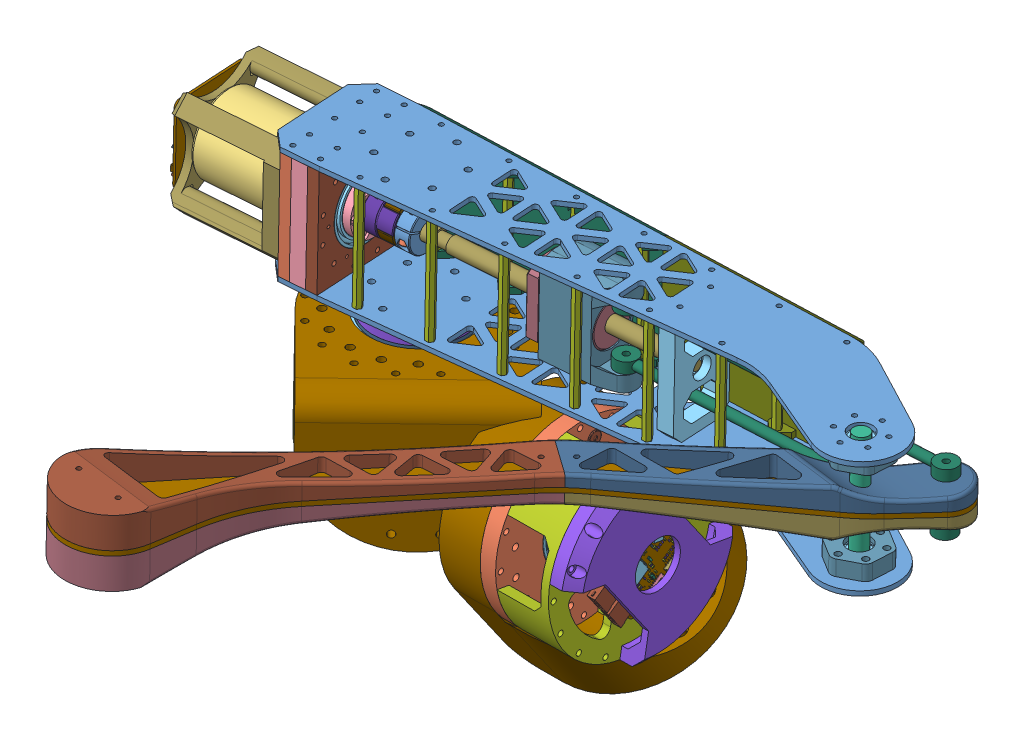
SolidWorks assembly Leg, configuration Default. Lengths in mm. (continued)
Components (placement in the parent): (continued)
- leg_cover-1: leg_cover [Default] at (234.1651 210.9123 294.9572) x (-0.000153 0.999777 -0.0211) z (0.036778 0.021091 0.999101) size (76 156.5 15.51)
- leg_cover_2-1: leg_cover_2 [Default] at (363.0778 210.8319 290.2135) x (-0.000153 0.999777 -0.0211) z (0.036778 0.021091 0.999101) size (76 129 15.51)
- Cycloidal _v3-1: Cycloidal _v3 [Default] at (201.9883 83.8715 287.662) x (0.007254 0.020702 0.999759) z (-0.999974 0 0.007256) size (173.36 87.57 173.15)
  - motor-X83008S.stp-1: motor-X83008S.stp [Default] at (3.9105 88.7742 94.1058) x (0.928336 0.00037 -0.371741) z (0.000399 -1 0) size (114.7 114.7 37.62) (hidden)
    - base.stp-1: base.stp [Default] at (42.0794 12.0269 46.7342) size (91.6 91.6 15.61)
    - stator.stp-1: stator.stp [Default] at (42.0794 12.0269 33.1342) x (0.08493 -0.996387 0) z (0 0 1) size (83 83 8)
    - coil.stp-1: coil.stp [Default] at (39.5332 41.8984 37.1342) x (0.996387 0.08493 0) z (-0.08493 0.996387 0) size (4.4 10.2 10.5)
    - coil.stp-2: coil.stp [Default] at (34.3848 41.0025 37.1342) x (0.966502 0.256661 0) z (-0.256661 0.966502 0) size (4.4 10.2 10.5)
    - coil.stp-3: coil.stp [Default] at (29.4701 39.2261 37.1342) x (0.90725 0.420593 0) z (-0.420593 0.90725 0) size (4.4 10.2 10.5)
    - coil.stp-4: coil.stp [Default] at (24.9386 36.6233 37.1342) x (0.820431 0.571745 0) z (-0.571745 0.820431 0) size (4.4 10.2 10.5)
    - coil.stp-5: coil.stp [Default] at (20.9279 33.2732 37.1342) x (0.708685 0.705525 0) z (-0.705525 0.708685 0) size (4.4 10.2 10.5)
    - coil.stp-6: coil.stp [Default] at (17.5599 29.2775 37.1342) x (0.575405 0.817869 0) z (-0.817869 0.575405 0) size (4.4 10.2 10.5)
    - coil.stp-7: coil.stp [Default] at (14.9368 24.7576 37.1342) x (0.424642 0.905361 0) z (-0.905361 0.424642 0) size (4.4 10.2 10.5)
    - coil.stp-8: coil.stp [Default] at (13.1385 19.8509 37.1342) x (0.260976 0.965345 0) z (-0.965345 0.260976 0) size (4.4 10.2 10.5)
    - coil.stp-9: coil.stp [Default] at (12.2196 14.7066 37.1342) x (0.089381 0.995998 0) z (-0.995998 0.089381 0) size (4.4 10.2 10.5)
    - coil.stp-10: coil.stp [Default] at (12.2079 9.4807 37.1342) x (-0.08493 0.996387 0) z (-0.996387 -0.08493 0) size (4.4 10.2 10.5)
    - coil.stp-11: coil.stp [Default] at (13.1039 4.3323 37.1342) x (-0.256661 0.966502 0) z (-0.966502 -0.256661 0) size (4.4 10.2 10.5)
    - coil.stp-12: coil.stp [Default] at (14.8802 -0.5824 37.1342) x (-0.420593 0.90725 0) z (-0.90725 -0.420593 0) size (4.4 10.2 10.5)
    - coil.stp-13: coil.stp [Default] at (17.483 -5.1139 37.1342) x (-0.571745 0.820431 0) z (-0.820431 -0.571745 0) size (4.4 10.2 10.5)
    - coil.stp-14: coil.stp [Default] at (20.8332 -9.1246 37.1342) x (-0.705525 0.708685 0) z (-0.708685 -0.705525 0) size (4.4 10.2 10.5)
    - coil.stp-15: coil.stp [Default] at (24.8289 -12.4926 37.1342) x (-0.817869 0.575405 0) z (-0.575405 -0.817869 0) size (4.4 10.2 10.5)
    - coil.stp-16: coil.stp [Default] at (29.3487 -15.1157 37.1342) x (-0.905361 0.424642 0) z (-0.424642 -0.905361 0) size (4.4 10.2 10.5)
    - coil.stp-17: coil.stp [Default] at (34.2554 -16.914 37.1342) x (-0.965345 0.260976 0) z (-0.260976 -0.965345 0) size (4.4 10.2 10.5)
    - coil.stp-18: coil.stp [Default] at (39.3998 -17.8329 37.1342) x (-0.995998 0.089381 0) z (-0.089381 -0.995998 0) size (4.4 10.2 10.5)
    - coil.stp-19: coil.stp [Default] at (44.6256 -17.8446 37.1342) x (-0.996387 -0.08493 0) z (0.08493 -0.996387 0) size (4.4 10.2 10.5)
    - coil.stp-20: coil.stp [Default] at (49.7741 -16.9486 37.1342) x (-0.966502 -0.256661 0) z (0.256661 -0.966502 0) size (4.4 10.2 10.5)
    - coil.stp-21: coil.stp [Default] at (54.6887 -15.1723 37.1342) x (-0.90725 -0.420593 0) z (0.420593 -0.90725 0) size (4.4 10.2 10.5)
    - coil.stp-22: coil.stp [Default] at (59.2202 -12.5695 37.1342) x (-0.820431 -0.571745 0) z (0.571745 -0.820431 0) size (4.4 10.2 10.5)
    - coil.stp-23: coil.stp [Default] at (63.2309 -9.2193 37.1342) x (-0.708685 -0.705525 0) z (0.705525 -0.708685 0) size (4.4 10.2 10.5)
    - coil.stp-24: coil.stp [Default] at (66.599 -5.2236 37.1342) x (-0.575405 -0.817869 0) z (0.817869 -0.575405 0) size (4.4 10.2 10.5)
    - coil.stp-25: coil.stp [Default] at (69.222 -0.7038 37.1342) x (-0.424642 -0.905361 0) z (0.905361 -0.424642 0) size (4.4 10.2 10.5)
    - coil.stp-26: coil.stp [Default] at (71.0203 4.2029 37.1342) x (-0.260976 -0.965345 0) z (0.965345 -0.260976 0) size (4.4 10.2 10.5)
    - coil.stp-27: coil.stp [Default] at (71.9392 9.3473 37.1342) x (-0.089381 -0.995998 0) z (0.995998 -0.089381 0) size (4.4 10.2 10.5)
    - coil.stp-28: coil.stp [Default] at (71.9509 14.5731 37.1342) x (0.08493 -0.996387 0) z (0.996387 0.08493 0) size (4.4 10.2 10.5)
    - coil.stp-29: coil.stp [Default] at (71.055 19.7216 37.1342) x (0.256661 -0.966502 0) z (0.966502 0.256661 0) size (4.4 10.2 10.5)
    - coil.stp-30: coil.stp [Default] at (69.2786 24.6362 37.1342) x (0.420593 -0.90725 0) z (0.90725 0.420593 0) size (4.4 10.2 10.5)
    - coil.stp-31: coil.stp [Default] at (66.6758 29.1677 37.1342) x (0.571745 -0.820431 0) z (0.820431 0.571745 0) size (4.4 10.2 10.5)
    - coil.stp-32: coil.stp [Default] at (63.3257 33.1785 37.1342) x (0.705525 -0.708685 0) z (0.708685 0.705525 0) size (4.4 10.2 10.5)
    - coil.stp-33: coil.stp [Default] at (59.33 36.5465 37.1342) x (0.817869 -0.575405 0) z (0.575405 0.817869 0) size (4.4 10.2 10.5)
    - coil.stp-34: coil.stp [Default] at (54.8101 39.1695 37.1342) x (0.905361 -0.424642 0) z (0.424642 0.905361 0) size (4.4 10.2 10.5)
    - coil.stp-35: coil.stp [Default] at (49.9034 40.9678 37.1342) x (0.965345 -0.260976 0) z (0.260976 0.965345 0) size (4.4 10.2 10.5)
    - coil.stp-36: coil.stp [Default] at (44.759 41.8868 37.1342) x (0.995998 -0.089381 0) z (0.089381 0.995998 0) size (4.4 10.2 10.5)
    - rotor.stp-1: rotor.stp [Default] at (42.0794 12.0269 42.1342) x (-0.293442 0.955977 0) z (0 0 -1) size (91.8 91.8 12)
    - outrunner.stp-1: outrunner.stp [Default] at (42.0794 12.0269 30.1342) x (-0.254711 0.967017 0) z (-0.967017 -0.254711 0) size (91.8 17.01 91.8)
    - screw-mount.stp-1: screw-mount.stp [Default] at (38.1314 27.0157 27.1342) x (1 0 0) z (0 0 -1) size (7 7 6.5)
    - screw-mount.stp-2: screw-mount.stp [Default] at (27.0906 8.0789 27.1342) x (1 0 0) z (0 0 -1) size (7 7 6.5)
    - screw-mount.stp-3: screw-mount.stp [Default] at (57.0682 15.9749 27.1342) x (1 0 0) z (0 0 -1) size (7 7 6.5)
    - screw-mount.stp-4: screw-mount.stp [Default] at (46.0274 -2.9618 27.1342) x (1 0 0) z (0 0 -1) size (7 7 6.5)
    - 6702ZZ-bearing-15x21x4.stp-1: 6702ZZ-bearing-15x21x4.stp [Default] at (42.0794 12.0269 43.7342) x (1 0 0) z (0 -1 0) size (21 4 21)
    - 6702ZZ-bearing-15x21x4.stp-2: 6702ZZ-bearing-15x21x4.stp [Default] at (42.0794 12.0269 35.1342) x (1 0 0) z (0 1 0) size (21 4 21)
    - shaft.stp-1: shaft.stp [Default] at (42.0794 12.0269 20.1342) size (16 16 31.6)
    - fix-screw.stp-1: fix-screw.stp [Default] at (42.0794 12.0269 51.7342) x (1 0 0) z (0 0 -1) size (19.67 18.96 12.02)
  - Base_Plate-1: Base_Plate [Default] at (47.4533 68.6574 89.6282) x (-0.992404 -0.000396 0.123023) z (-0.123023 -0.000049 -0.992404) size (39.8 11 39.8)
  - Eccentric_Shaft-1: Eccentric_Shaft [Default] at (60.4961 73.3217 80.3225) x (0.123023 0.000049 0.992404) z (-0.992404 -0.000396 0.123023) size (20 17 17)
    - Eccentric_Shaft_bot-1: Eccentric_Shaft_bot [Default] at (7.6302 12.3409 14.0904) x (1 0 0) z (0 0 -1) size (17 6 17)
    - Eccentric_Shaft_bot-2: Eccentric_Shaft_bot [Default] at (7.6302 12.3409 14.0904) x (-1 0 0) z (0 0 -1) size (17 6 17)
    - Eccentric_Shaft_top-1: Eccentric_Shaft_top [Default] at (7.6302 18.3409 14.0904) x (-1 0 0) z (0 0 -1) size (17 5 17)
  - radial ball bearing_68_iso-39: radial ball bearing_68_iso [ISO 15 RBB - 1860 - 32,SI,NC,32_68] at (47.4409 99.6574 89.6282) x (0.000399 -1 0) z (-0.546908 -0.000218 0.837193) size (10 78 78)
  - radial ball bearing_68_iso-40: radial ball bearing_68_iso [ISO 15 RBB - 1840 - 32,SI,NC,32_68] at (47.4516 72.9574 89.6282) x (-0.000399 1 0) z (0.001003 0 0.999999) size (7 52 52)
  - Base_plate_2-1: Base_plate_2 [Default] at (47.4529 69.6574 89.6282) x (0.712755 0.000284 -0.701413) z (0.701413 0.00028 0.712755) size (115 10 115)
  - m13_bearing-31: m13_bearing [Default] at (-10.4263 95.4017 67.196) x (0.227678 0.000091 0.973736) z (0.973736 0.000388 -0.227678) size (13 16 13)
    - m6-1: m6 [Default] at (8.4921 2.5508 14.8914) size (6 16 6)
    - radial ball bearing_68_iso-1: radial ball bearing_68_iso [ISO 15 RBB - 286 - 10,SI,NC,10_68] at (8.4921 16.0508 14.8914) x (0 1 0) z (0 0 1) size (5 13 13)
    - radial ball bearing_68_iso-2: radial ball bearing_68_iso [ISO 15 RBB - 286 - 10,SI,NC,10_68] at (8.4921 11.0508 14.8914) x (0 1 0) z (0 0 1) size (5 13 13)
  - m13_bearing-32: m13_bearing [Default] at (-13.9908 98.1837 84.3887) x (0.227678 0.000091 0.973736) z (0.973736 0.000388 -0.227678) size (13 16 13)
    - m6-1: m6 [Default] at (8.4921 2.5508 14.8914) size (6 16 6)
    - radial ball bearing_68_iso-1: radial ball bearing_68_iso [ISO 15 RBB - 286 - 10,SI,NC,10_68] at (8.4921 16.0508 14.8914) x (0 1 0) z (0 0 1) size (5 13 13)
    - radial ball bearing_68_iso-2: radial ball bearing_68_iso [ISO 15 RBB - 286 - 10,SI,NC,10_68] at (8.4921 11.0508 14.8914) x (0 1 0) z (0 0 1) size (5 13 13)
  - m13_bearing-34: m13_bearing [Default] at (13.4541 98.1947 126.1847) x (0.227678 0.000091 0.973736) z (0.973736 0.000388 -0.227678) size (13 16 13)
    - m6-1: m6 [Default] at (8.4921 2.5508 14.8914) size (6 16 6)
    - radial ball bearing_68_iso-1: radial ball bearing_68_iso [ISO 15 RBB - 286 - 10,SI,NC,10_68] at (8.4921 16.0508 14.8914) x (0 1 0) z (0 0 1) size (5 13 13)
    - radial ball bearing_68_iso-2: radial ball bearing_68_iso [ISO 15 RBB - 286 - 10,SI,NC,10_68] at (8.4921 11.0508 14.8914) x (0 1 0) z (0 0 1) size (5 13 13)
  - m13_bearing-35: m13_bearing [Default] at (-1.0662 98.1889 116.3132) x (0.227678 0.000091 0.973736) z (0.973736 0.000388 -0.227678) size (13 16 13)
    - m6-1: m6 [Default] at (8.4921 2.5508 14.8914) size (6 16 6)
    - radial ball bearing_68_iso-1: radial ball bearing_68_iso [ISO 15 RBB - 286 - 10,SI,NC,10_68] at (8.4921 16.0508 14.8914) x (0 1 0) z (0 0 1) size (5 13 13)
    - radial ball bearing_68_iso-2: radial ball bearing_68_iso [ISO 15 RBB - 286 - 10,SI,NC,10_68] at (8.4921 11.0508 14.8914) x (0 1 0) z (0 0 1) size (5 13 13)
  - m13_bearing-36: m13_bearing [Default] at (-10.7036 98.185 101.6364) x (0.227678 0.000091 0.973736) z (0.973736 0.000388 -0.227678) size (13 16 13)
    - m6-1: m6 [Default] at (8.4921 2.5508 14.8914) size (6 16 6)
    - radial ball bearing_68_iso-1: radial ball bearing_68_iso [ISO 15 RBB - 286 - 10,SI,NC,10_68] at (8.4921 16.0508 14.8914) x (0 1 0) z (0 0 1) size (5 13 13)
    - radial ball bearing_68_iso-2: radial ball bearing_68_iso [ISO 15 RBB - 286 - 10,SI,NC,10_68] at (8.4921 11.0508 14.8914) x (0 1 0) z (0 0 1) size (5 13 13)
  - m13_bearing-1: m13_bearing [Default] at (-0.4494 98.1891 62.778) x (0.736525 0.000294 0.676411) z (0.676411 0.00027 -0.736525) size (13 16 13)
    - m6-1: m6 [Default] at (8.4921 2.5508 14.8914) size (6 16 6)
    - radial ball bearing_68_iso-1: radial ball bearing_68_iso [ISO 15 RBB - 286 - 10,SI,NC,10_68] at (8.4921 16.0508 14.8914) x (0 1 0) z (0 0 1) size (5 13 13)
    - radial ball bearing_68_iso-2: radial ball bearing_68_iso [ISO 15 RBB - 286 - 10,SI,NC,10_68] at (8.4921 11.0508 14.8914) x (0 1 0) z (0 0 1) size (5 13 13)
  - m13_bearing-2: m13_bearing [Default] at (48.5236 98.2087 124.7001) x (0.120271 0.000048 0.992741) z (0.992741 0.000396 -0.120271) size (13 16 13)
    - m6-1: m6 [Default] at (8.4921 2.5508 14.8914) size (6 16 6)
    - radial ball bearing_68_iso-1: radial ball bearing_68_iso [ISO 15 RBB - 286 - 10,SI,NC,10_68] at (8.4921 16.0508 14.8914) x (0 1 0) z (0 0 1) size (5 13 13)
    - radial ball bearing_68_iso-2: radial ball bearing_68_iso [ISO 15 RBB - 286 - 10,SI,NC,10_68] at (8.4921 11.0508 14.8914) x (0 1 0) z (0 0 1) size (5 13 13)
  - m13_bearing-3: m13_bearing [Default] at (32.5019 98.2023 52.3604) x (0.833889 0.000333 0.551933) z (0.551932 0.00022 -0.833889) size (13 16 13)
    - m6-1: m6 [Default] at (8.4921 2.5508 14.8914) size (6 16 6)
    - radial ball bearing_68_iso-1: radial ball bearing_68_iso [ISO 15 RBB - 286 - 10,SI,NC,10_68] at (8.4921 16.0508 14.8914) x (0 1 0) z (0 0 1) size (5 13 13)
    - radial ball bearing_68_iso-2: radial ball bearing_68_iso [ISO 15 RBB - 286 - 10,SI,NC,10_68] at (8.4921 11.0508 14.8914) x (0 1 0) z (0 0 1) size (5 13 13)
  - m13_bearing-4: m13_bearing [Default] at (77.3632 98.2202 81.8307) x (0.022268 0.000009 0.999752) z (0.999752 0.000399 -0.022268) size (13 16 13)
    - m6-1: m6 [Default] at (8.4921 2.5508 14.8914) size (6 16 6)
    - radial ball bearing_68_iso-1: radial ball bearing_68_iso [ISO 15 RBB - 286 - 10,SI,NC,10_68] at (8.4921 16.0508 14.8914) x (0 1 0) z (0 0 1) size (5 13 13)
    - radial ball bearing_68_iso-2: radial ball bearing_68_iso [ISO 15 RBB - 286 - 10,SI,NC,10_68] at (8.4921 11.0508 14.8914) x (0 1 0) z (0 0 1) size (5 13 13)
  - m13_bearing-5: m13_bearing [Default] at (73.5091 98.2186 99.5852) x (0.059133 0.000024 0.99825) z (0.99825 0.000398 -0.059133) size (13 16 13)
    - m6-1: m6 [Default] at (8.4921 2.5508 14.8914) size (6 16 6)
    - radial ball bearing_68_iso-1: radial ball bearing_68_iso [ISO 15 RBB - 286 - 10,SI,NC,10_68] at (8.4921 16.0508 14.8914) x (0 1 0) z (0 0 1) size (5 13 13)
    - radial ball bearing_68_iso-2: radial ball bearing_68_iso [ISO 15 RBB - 286 - 10,SI,NC,10_68] at (8.4921 11.0508 14.8914) x (0 1 0) z (0 0 1) size (5 13 13)
  - m13_bearing-6: m13_bearing [Default] at (13.4333 98.1947 47.0643) x (0.451561 0.00018 0.89224) z (0.89224 0.000356 -0.451561) size (13 16 13)
    - m6-1: m6 [Default] at (8.4921 2.5508 14.8914) size (6 16 6)
    - radial ball bearing_68_iso-1: radial ball bearing_68_iso [ISO 15 RBB - 286 - 10,SI,NC,10_68] at (8.4921 16.0508 14.8914) x (0 1 0) z (0 0 1) size (5 13 13)
    - radial ball bearing_68_iso-2: radial ball bearing_68_iso [ISO 15 RBB - 286 - 10,SI,NC,10_68] at (8.4921 11.0508 14.8914) x (0 1 0) z (0 0 1) size (5 13 13)
  - m13_bearing-7: m13_bearing [Default] at (57.1526 98.2121 32.9496) x (-0.545813 -0.000218 0.837907) z (0.837907 0.000334 0.545813) size (13 16 13)
    - m6-1: m6 [Default] at (8.4921 2.5508 14.8914) size (6 16 6)
    - radial ball bearing_68_iso-1: radial ball bearing_68_iso [ISO 15 RBB - 286 - 10,SI,NC,10_68] at (8.4921 16.0508 14.8914) x (0 1 0) z (0 0 1) size (5 13 13)
    - radial ball bearing_68_iso-2: radial ball bearing_68_iso [ISO 15 RBB - 286 - 10,SI,NC,10_68] at (8.4921 11.0508 14.8914) x (0 1 0) z (0 0 1) size (5 13 13)
  - m13_bearing-8: m13_bearing [Default] at (73.1034 98.2185 66.7178) x (0.158553 0.000063 0.98735) z (0.98735 0.000394 -0.158553) size (13 16 13)
    - m6-1: m6 [Default] at (8.4921 2.5508 14.8914) size (6 16 6)
    - radial ball bearing_68_iso-1: radial ball bearing_68_iso [ISO 15 RBB - 286 - 10,SI,NC,10_68] at (8.4921 16.0508 14.8914) x (0 1 0) z (0 0 1) size (5 13 13)
    - radial ball bearing_68_iso-2: radial ball bearing_68_iso [ISO 15 RBB - 286 - 10,SI,NC,10_68] at (8.4921 11.0508 14.8914) x (0 1 0) z (0 0 1) size (5 13 13)
  - m13_bearing-9: m13_bearing [Default] at (74.5316 98.219 41.6624) x (-0.687134 -0.000274 0.72653) z (0.72653 0.00029 0.687134) size (13 16 13)
    - m6-1: m6 [Default] at (8.4921 2.5508 14.8914) size (6 16 6)
    - radial ball bearing_68_iso-1: radial ball bearing_68_iso [ISO 15 RBB - 286 - 10,SI,NC,10_68] at (8.4921 16.0508 14.8914) x (0 1 0) z (0 0 1) size (5 13 13)
    - radial ball bearing_68_iso-2: radial ball bearing_68_iso [ISO 15 RBB - 286 - 10,SI,NC,10_68] at (8.4921 11.0508 14.8914) x (0 1 0) z (0 0 1) size (5 13 13)
  - m13_bearing-11: m13_bearing [Default] at (30.0113 98.2013 136.2104) x (0.57351 0.000229 0.819198) z (0.819198 0.000327 -0.57351) size (13 16 13)
    - m6-1: m6 [Default] at (8.4921 2.5508 14.8914) size (6 16 6)
    - radial ball bearing_68_iso-1: radial ball bearing_68_iso [ISO 15 RBB - 286 - 10,SI,NC,10_68] at (8.4921 16.0508 14.8914) x (0 1 0) z (0 0 1) size (5 13 13)
    - radial ball bearing_68_iso-2: radial ball bearing_68_iso [ISO 15 RBB - 286 - 10,SI,NC,10_68] at (8.4921 11.0508 14.8914) x (0 1 0) z (0 0 1) size (5 13 13)
  - m13_bearing-12: m13_bearing [Default] at (62.5932 98.2143 116.7506) x (0.22335 0.000089 0.974738) z (0.974738 0.000389 -0.22335) size (13 16 13)
    - m6-1: m6 [Default] at (8.4921 2.5508 14.8914) size (6 16 6)
    - radial ball bearing_68_iso-1: radial ball bearing_68_iso [ISO 15 RBB - 286 - 10,SI,NC,10_68] at (8.4921 16.0508 14.8914) x (0 1 0) z (0 0 1) size (5 13 13)
    - radial ball bearing_68_iso-2: radial ball bearing_68_iso [ISO 15 RBB - 286 - 10,SI,NC,10_68] at (8.4921 11.0508 14.8914) x (0 1 0) z (0 0 1) size (5 13 13)
  - M3x4x4.2_brass_insert-22: M3x4x4.2_brass_insert [Default] at (43.4837 68.6558 90.1203) x (0.984609 0.000393 -0.174769) z (0.174769 0.00007 0.984609) size (4 4 4)
  - M3x4x4.2_brass_insert-23: M3x4x4.2_brass_insert [Default] at (51.4229 68.659 89.1361) x (0.984609 0.000393 -0.174769) z (0.174769 0.00007 0.984609) size (4 4 4)
  - radial ball bearing_68_iso-44: radial ball bearing_68_iso [ISO 15 RBB - 1715 - 26,SI,NC,26_68] at (47.2636 81.6573 88.1396) x (0.000399 -1 0) z (0.171535 0.000068 0.985178) size (4 21 21)
  - radial ball bearing_68_iso-45: radial ball bearing_68_iso [ISO 15 RBB - 1715 - 26,SI,NC,26_68] at (47.4429 94.6574 89.6282) x (0.000399 -1 0) z (0.819169 0.000327 0.573552) size (4 21 21)
  - radial ball bearing_68_iso-46: radial ball bearing_68_iso [ISO 15 RBB - 1715 - 26,SI,NC,26_68] at (47.6295 89.6575 91.1168) x (-0.000399 1 0) z (0 0 1) size (4 21 21)
  - foc-motor-controller.step-1: foc-motor-controller.step [Default] at (47.4677 32.6574 89.6282) x (0.701413 0.00028 0.712755) z (0.000399 -1 0) size (57.23 50 8.13)
    - RTA0040B.step-1: RTA0040B.step [Default] at (12.5014 -1.6986 1.595) x (-0.707107 -0.707107 0) z (0 0 1) size (6 6 1)
      - FRAME.step-1: FRAME.step [Default] x (1 0 0) z (0 -1 0) size (6 0.2 6)
        - SOLID.step-1: SOLID.step [Default] at origin size (0.4 0.2 0.22)
        - SOLID-0.step-1: SOLID-0.step [Default] at origin size (0.4 0.2 0.22)
        - SOLID-1.step-1: SOLID-1.step [Default] at origin size (0.4 0.2 0.22)
        - SOLID-2.step-1: SOLID-2.step [Default] at origin size (0.4 0.2 0.22)
        - SOLID-3.step-1: SOLID-3.step [Default] at origin size (0.4 0.2 0.22)
        - SOLID-4.step-1: SOLID-4.step [Default] at origin size (0.4 0.2 0.22)
        - SOLID-5.step-1: SOLID-5.step [Default] at origin size (0.4 0.2 0.22)
        - SOLID-6.step-1: SOLID-6.step [Default] at origin size (0.4 0.2 0.22)
        - SOLID-7.step-1: SOLID-7.step [Default] at origin size (0.4 0.2 0.22)
        - SOLID-8.step-1: SOLID-8.step [Default] at origin size (0.4 0.2 0.22)
        - SOLID-9.step-1: SOLID-9.step [Default] at origin size (0.22 0.2 0.4)
        - SOLID-10.step-1: SOLID-10.step [Default] at origin size (0.22 0.2 0.4)
        - SOLID-11.step-1: SOLID-11.step [Default] at origin size (0.22 0.2 0.4)
        - SOLID-12.step-1: SOLID-12.step [Default] at origin size (0.22 0.2 0.4)
        - SOLID-13.step-1: SOLID-13.step [Default] at origin size (0.22 0.2 0.4)
        - SOLID-14.step-1: SOLID-14.step [Default] at origin size (0.22 0.2 0.4)
        - SOLID-15.step-1: SOLID-15.step [Default] at origin size (0.22 0.2 0.4)
        - SOLID-16.step-1: SOLID-16.step [Default] at origin size (0.22 0.2 0.4)
        - SOLID-17.step-1: SOLID-17.step [Default] at origin size (4.15 0.2 4.15)
        - SOLID-18.step-1: SOLID-18.step [Default] at origin size (0.28 0.1 0.28)
        - SOLID-19.step-1: SOLID-19.step [Default] at origin size (0.28 0.1 0.28)
        - SOLID-20.step-1: SOLID-20.step [Default] at origin size (0.28 0.1 0.28)
        - SOLID-21.step-1: SOLID-21.step [Default] at origin size (0.28 0.1 0.28)
        - SOLID-22.step-1: SOLID-22.step [Default] at origin size (0.4 0.2 0.22)
        - SOLID-23.step-1: SOLID-23.step [Default] at origin size (0.4 0.2 0.22)
        - SOLID-24.step-1: SOLID-24.step [Default] at origin size (0.4 0.2 0.22)
        - SOLID-25.step-1: SOLID-25.step [Default] at origin size (0.4 0.2 0.22)
        - SOLID-26.step-1: SOLID-26.step [Default] at origin size (0.4 0.2 0.22)
        - SOLID-27.step-1: SOLID-27.step [Default] at origin size (0.4 0.2 0.22)
        - SOLID-28.step-1: SOLID-28.step [Default] at origin size (0.4 0.2 0.22)
        - SOLID-29.step-1: SOLID-29.step [Default] at origin size (0.4 0.2 0.22)
        - SOLID-30.step-1: SOLID-30.step [Default] at origin size (0.4 0.2 0.22)
        - SOLID-31.step-1: SOLID-31.step [Default] at origin size (0.4 0.2 0.22)
        - SOLID-32.step-1: SOLID-32.step [Default] at origin size (0.22 0.2 0.4)
        - SOLID-33.step-1: SOLID-33.step [Default] at origin size (0.22 0.2 0.4)
        - SOLID-34.step-1: SOLID-34.step [Default] at origin size (0.22 0.2 0.4)
        - SOLID-35.step-1: SOLID-35.step [Default] at origin size (0.22 0.2 0.4)
        - SOLID-36.step-1: SOLID-36.step [Default] at origin size (0.22 0.2 0.4)
        - SOLID-37.step-1: SOLID-37.step [Default] at origin size (0.22 0.2 0.4)
        - SOLID-38.step-1: SOLID-38.step [Default] at origin size (0.22 0.2 0.4)
        - SOLID-39.step-1: SOLID-39.step [Default] at origin size (0.22 0.2 0.4)
        - SOLID-40.step-1: SOLID-40.step [Default] at origin size (0.22 0.2 0.4)
        - SOLID-41.step-1: SOLID-41.step [Default] at origin size (0.22 0.2 0.4)
        - SOLID-42.step-1: SOLID-42.step [Default] at origin size (0.22 0.2 0.4)
        - SOLID-43.step-1: SOLID-43.step [Default] at origin size (0.22 0.2 0.4)
      - BODY.step-1: BODY.step [Default] at (0 0 0.025) x (1 0 0) z (0 -1 0) size (6 0.97 6)
    - Resonator_SMD_Murata_CSTxExxV-3Pin_3.0x1.1mm.step-1: Resonator_SMD_Murata_CSTxExxV-3Pin_3.0x1.1mm.step [Default] at (1.8 -7 1.595) x (0 1 0) z (0 0 1) size (3.2 1.35 0.9)
    - C_0603_1608Metric.step-1: C_0603_1608Metric.step [Default] at (6.2 -16.8 1.595) x (0 -1 0) z (0 0 1) size (1.6 0.8 0.8)
    - R_0603_1608Metric.step-1: R_0603_1608Metric.step [Default] at (11.8 -7.375 1.595) x (0 1 0) z (0 0 1) size (1.6 0.8 0.45)
    - R_0603_1608Metric.step-2: R_0603_1608Metric.step [Default] at (13.8 -16.8 1.595) x (0 1 0) z (0 0 1) size (1.6 0.8 0.45)
    - R_0603_1608Metric.step-3: R_0603_1608Metric.step [Default] at (18.1 -5.36 1.595) size (1.6 0.8 0.45)
    - C_0603_1608Metric.step-2: C_0603_1608Metric.step [Default] at (2.6 -0.5 1.595) x (0 -1 0) z (0 0 1) size (1.6 0.8 0.8)
    - R_0603_1608Metric.step-4: R_0603_1608Metric.step [Default] at (14.6 -11.3 1.595) x (0 1 0) z (0 0 1) size (1.6 0.8 0.45)
    - L_APV_ANR4020.step-1: L_APV_ANR4020.step [Default] at (22.3 -13.7 1.595) x (0 -1 0) z (0 0 1) size (4.02 4 2)
    - C_0603_1608Metric.step-3: C_0603_1608Metric.step [Default] at (0.3 -12.6 1.595) x (-1 0 0) z (0 0 1) size (1.6 0.8 0.8)
    - C_1206_3216Metric.step-1: C_1206_3216Metric.step [Default] at (15.7 11 1.595) x (0 1 0) z (0 0 1) size (3.2 1.6 1.6)
    - C_0603_1608Metric.step-4: C_0603_1608Metric.step [Default] at (0.3 -9.6 1.595) size (1.6 0.8 0.8)
    - R_0603_1608Metric.step-5: R_0603_1608Metric.step [Default] at (12.3 -16.8 1.595) x (0 1 0) z (0 0 1) size (1.6 0.8 0.45)
    - C_0603_1608Metric.step-5: C_0603_1608Metric.step [Default] at (-0.3 -16.6 1.595) x (0 1 0) z (0 0 1) size (1.6 0.8 0.8)
    - R_0603_1608Metric.step-6: R_0603_1608Metric.step [Default] at (10.9 4.1 1.595) size (1.6 0.8 0.45)
    - C_1206_3216Metric.step-2: C_1206_3216Metric.step [Default] at (6.3 11 1.595) x (0 1 0) z (0 0 1) size (3.2 1.6 1.6)
    - XT30PW_2_2_-M.G.B.step-1: XT30PW_2_2_-M.G.B.step [Default] at (-20.5 9.5 1.595) x (0 -1 0) z (-1 0 0) size (15.5 7.1 12.53)
    - R_0603_1608Metric.step-7: R_0603_1608Metric.step [Default] at (0.3 -11.1 1.595) size (1.6 0.8 0.45)
    - C_0603_1608Metric.step-6: C_0603_1608Metric.step [Default] at (19 -0.4 1.595) x (-0.707107 -0.707107 0) z (0 0 1) size (1.6 0.8 0.8)
    - C_1206_3216Metric.step-3: C_1206_3216Metric.step [Default] at (13.3 11 1.595) x (0 1 0) z (0 0 1) size (3.2 1.6 1.6)
    - R_0603_1608Metric.step-8: R_0603_1608Metric.step [Default] at (10.2 -7.375 1.595) x (0 -1 0) z (0 0 1) size (1.6 0.8 0.45)
    - JST_GH_SM08B-GHS-TB_1x08-1MP_P1.25mm_Horizontal.step-1: JST_GH_SM08B-GHS-TB_1x08-1MP_P1.25mm_Horizontal.step [Default] at (10 -22 1.595) size (13.25 4.95 4.25)
    - C_1206_3216Metric.step-4: C_1206_3216Metric.step [Default] at (-12.3 11 1.595) x (0 1 0) z (0 0 1) size (3.2 1.6 1.6)
    - JST_GH_SM06B-GHS-TB_1x06-1MP_P1.25mm_Horizontal.step-1: JST_GH_SM06B-GHS-TB_1x06-1MP_P1.25mm_Horizontal.step [Default] at (-4.3 -22 1.595) size (10.75 4.95 4.25)
    - C_0603_1608Metric.step-7: C_0603_1608Metric.step [Default] at (7.3 -4.5 1.595) x (-1 0 0) z (0 0 1) size (1.6 0.8 0.8)
    - R_0603_1608Metric.step-9: R_0603_1608Metric.step [Default] at (18.1 -3.86 1.595) x (-1 0 0) z (0 0 1) size (1.6 0.8 0.45)
    - C_1206_3216Metric.step-5: C_1206_3216Metric.step [Default] at (22.6794 -1.2206 1.595) x (0.707107 -0.707107 0) z (0 0 1) size (3.2 1.6 1.6)
    - R_Array_Convex_4x0402.step-1: R_Array_Convex_4x0402.step [Default] at (6.8 -2.5 1.595) size (1 2 0.35)
    - R_0603_1608Metric.step-10: R_0603_1608Metric.step [Default] at (7.7 -16.8 1.595) x (0 -1 0) z (0 0 1) size (1.6 0.8 0.45)
    - C_1206_3216Metric.step-6: C_1206_3216Metric.step [Default] at (8.7 11 1.595) x (0 1 0) z (0 0 1) size (3.2 1.6 1.6)
    - C_0603_1608Metric.step-8: C_0603_1608Metric.step [Default] at (16.1 -11.3 1.595) x (0 1 0) z (0 0 1) size (1.6 0.8 0.8)
    - SOT-23-5.step-1: SOT-23-5.step [Default] at (-3.1 -16.6 1.595) x (-1 0 0) z (0 0 1) size (2.8 2.9 1.55)
    - C_0603_1608Metric.step-9: C_0603_1608Metric.step [Default] at (17.8 -13.6 1.595) size (1.6 0.8 0.8)
    - R_0603_1608Metric.step-11: R_0603_1608Metric.step [Default] at (-11.5 -20.3875 1.595) x (0 -1 0) z (0 0 1) size (1.6 0.8 0.45)
    - C_0603_1608Metric.step-10: C_0603_1608Metric.step [Default] at (-12.4 2.3 1.595) x (0 1 0) z (0 0 1) size (1.6 0.8 0.8)
    - C_1206_3216Metric.step-7: C_1206_3216Metric.step [Default] at (18 11 1.595) x (0 1 0) z (0 0 1) size (3.2 1.6 1.6)
    - R_0603_1608Metric.step-12: R_0603_1608Metric.step [Default] at (-10.8105 -14.9971 1.595) x (-1 0 0) z (0 0 1) size (1.6 0.8 0.45)
    - C_0603_1608Metric.step-11: C_0603_1608Metric.step [Default] at (-13.8 -9.4 1.595) x (-1 0 0) z (0 0 1) size (1.6 0.8 0.8)
    - R_0603_1608Metric.step-13: R_0603_1608Metric.step [Default] at (-23.15 -14.5 1.595) x (-1 0 0) z (0 0 1) size (1.6 0.8 0.45)
    - C_0603_1608Metric.step-12: C_0603_1608Metric.step [Default] at (1.1 -0.2 1.595) x (0 1 0) z (0 0 1) size (1.6 0.8 0.8)
    - D_0805_2012Metric.step-1: D_0805_2012Metric.step [Default] at (22.9 -9.6 1.595) x (0 1 0) z (0 0 1) size (2 1.27 0.8)
    - C_0603_1608Metric.step-13: C_0603_1608Metric.step [Default] at (-7.8 3.775 1.595) x (0 -1 0) z (0 0 1) size (1.6 0.8 0.8)
    - R_0603_1608Metric.step-14: R_0603_1608Metric.step [Default] at (-6.4 -12.825 1.595) x (0 1 0) z (0 0 1) size (1.6 0.8 0.45)
    - L_0603_1608Metric.step-1: L_0603_1608Metric.step [Default] at (-10.1 3 1.595) size (1.6 0.8 0.8)
    - C_0603_1608Metric.step-14: C_0603_1608Metric.step [Default] at (17.9 0.7 1.595) x (-0.707107 -0.707107 0) z (0 0 1) size (1.6 0.8 0.8)
    - HVSSOP-10.step-1: HVSSOP-10.step [Default] at (18.6 -9.6 1.595) x (0 -1 0) z (-1 0 0) size (4.9 1.1 3)
    - C_0603_1608Metric.step-15: C_0603_1608Metric.step [Default] at (7.9 4.1 1.595) x (-1 0 0) z (0 0 1) size (1.6 0.8 0.8)
    - C_0603_1608Metric.step-16: C_0603_1608Metric.step [Default] at (21.1 -9.6 1.595) x (0 -1 0) z (0 0 1) size (1.6 0.8 0.8)
    - R_0603_1608Metric.step-15: R_0603_1608Metric.step [Default] at (-10.8105 -11.9971 1.595) x (-1 0 0) z (0 0 1) size (1.6 0.8 0.45)
    - R_0603_1608Metric.step-16: R_0603_1608Metric.step [Default] at (-18.2 -17.4 1.595) size (1.6 0.8 0.45)
    - C_1206_3216Metric.step-8: C_1206_3216Metric.step [Default] at (-3 11 1.595) x (0 1 0) z (0 0 1) size (3.2 1.6 1.6)
    - R_0603_1608Metric.step-17: R_0603_1608Metric.step [Default] at (-16.9 -20.4 1.595) x (0 -1 0) z (0 0 1) size (1.6 0.8 0.45)
    - R_0603_1608Metric.step-18: R_0603_1608Metric.step [Default] at (-13.3 -20.3875 1.595) x (0 -1 0) z (0 0 1) size (1.6 0.8 0.45)
    - R_0603_1608Metric.step-19: R_0603_1608Metric.step [Default] at (-15.1 -20.3875 1.595) x (0 -1 0) z (0 0 1) size (1.6 0.8 0.45)
    - C_0603_1608Metric.step-17: C_0603_1608Metric.step [Default] at (15.5 -14.4 1.595) x (0 -1 0) z (0 0 1) size (1.6 0.8 0.8)
    - LED_0603_1608Metric.step-1: LED_0603_1608Metric.step [Default] at (-11.5 -23.3875 1.595) x (0 1 0) z (0 0 1) size (1.6 0.8 1.1)
    - C_0805_2012Metric.step-1: C_0805_2012Metric.step [Default] at (19.95 -17 1.595) size (2 1.25 1.25)
    - D_SMB.step-1: D_SMB.step [Default] at (-16.5 11.208 1.595) x (0 -1 0) z (0 0 1) size (5.3 3.55 2.15)
    - C_1206_3216Metric.step-9: C_1206_3216Metric.step [Default] at (-5.3 11 1.595) x (0 1 0) z (0 0 1) size (3.2 1.6 1.6)
    - XT30PW_2_2_-M.G.B.step-2: XT30PW_2_2_-M.G.B.step [Default] at (-20.5 -6.5 1.595) x (0 -1 0) z (-1 0 0) size (15.5 7.1 12.53)
    - C_1206_3216Metric.step-10: C_1206_3216Metric.step [Default] at (1.7 11 1.595) x (0 1 0) z (0 0 1) size (3.2 1.6 1.6)
    - C_1206_3216Metric.step-11: C_1206_3216Metric.step [Default] at (11 11 1.595) x (0 1 0) z (0 0 1) size (3.2 1.6 1.6)
    - C_0603_1608Metric.step-18: C_0603_1608Metric.step [Default] at (-6.3 3.775 1.595) x (0 -1 0) z (0 0 1) size (1.6 0.8 0.8)
    - C_0603_1608Metric.step-19: C_0603_1608Metric.step [Default] at (16.8686 1.7314 1.595) x (0.707107 0.707107 0) z (0 0 1) size (1.6 0.8 0.8)
    - C_0603_1608Metric.step-20: C_0603_1608Metric.step [Default] at (-15.0105 -11.1 1.595) size (1.6 0.8 0.8)
    - C_1206_3216Metric.step-12: C_1206_3216Metric.step [Default] at (-7.7 11 1.595) x (0 1 0) z (0 0 1) size (3.2 1.6 1.6)
    - C_0603_1608Metric.step-21: C_0603_1608Metric.step [Default] at (-18.2 -15.8 1.595) size (1.6 0.8 0.8)
    - C_0603_1608Metric.step-22: C_0603_1608Metric.step [Default] at (-2.1 -11.3 1.595) x (0 -1 0) z (0 0 1) size (1.6 0.8 0.8)
    - C_0603_1608Metric.step-23: C_0603_1608Metric.step [Default] at (-10.8105 -13.4971 1.595) size (1.6 0.8 0.8)
    - C_1206_3216Metric.step-13: C_1206_3216Metric.step [Default] at (4 11 1.595) x (0 1 0) z (0 0 1) size (3.2 1.6 1.6)
    - R_0603_1608Metric.step-20: R_0603_1608Metric.step [Default] at (16 -17.8 1.595) x (0 1 0) z (0 0 1) size (1.6 0.8 0.45)
    - Texas_S-PVSON-N8.step-1: Texas_S-PVSON-N8.step [Default] at (-14.4105 -13.7 1.595) x (-1 0 0) z (0 0 1) size (3 2.98 0.92)
    - C_1206_3216Metric.step-14: C_1206_3216Metric.step [Default] at (21 -2.9 1.595) x (0.707107 -0.707107 0) z (0 0 1) size (3.2 1.6 1.6)
    - C_0603_1608Metric.step-24: C_0603_1608Metric.step [Default] at (-5.9 -16.6 1.595) x (0 1 0) z (0 0 1) size (1.6 0.8 0.8)
    - C_0603_1608Metric.step-25: C_0603_1608Metric.step [Default] at (-3.1 -14.1 1.595) size (1.6 0.8 0.8)
    - R_0603_1608Metric.step-21: R_0603_1608Metric.step [Default] at (7.2 -7.375 1.595) x (0 -1 0) z (0 0 1) size (1.6 0.8 0.45)
    - C_1206_3216Metric.step-15: C_1206_3216Metric.step [Default] at (-0.7 11 1.595) x (0 1 0) z (0 0 1) size (3.2 1.6 1.6)
    - LQFP-64_10x10mm_P0.5mm.step-1: LQFP-64_10x10mm_P0.5mm.step [Default] at (-7 -4.5 1.595) x (-1 0 0) z (0 0 1) size (12 12 1.5)
    - C_0805_2012Metric.step-2: C_0805_2012Metric.step [Default] at (23.35 -17 1.595) x (-1 0 0) z (0 0 1) size (2 1.25 1.25)
    - C_0603_1608Metric.step-26: C_0603_1608Metric.step [Default] at (10.8 -16.8 1.595) x (0 -1 0) z (0 0 1) size (1.6 0.8 0.8)
    - R_0603_1608Metric.step-22: R_0603_1608Metric.step [Default] at (17.5 -17.8 1.595) x (0 -1 0) z (0 0 1) size (1.6 0.8 0.45)
    - C_1206_3216Metric.step-16: C_1206_3216Metric.step [Default] at (20.3 11 1.595) x (0 1 0) z (0 0 1) size (3.2 1.6 1.6)
    - R_0603_1608Metric.step-23: R_0603_1608Metric.step [Default] at (9.2 -16.8 1.595) x (0 -1 0) z (0 0 1) size (1.6 0.8 0.45)
    - C_1206_3216Metric.step-17: C_1206_3216Metric.step [Default] at (-10 11 1.595) x (0 1 0) z (0 0 1) size (3.2 1.6 1.6)
    - R_0603_1608Metric.step-24: R_0603_1608Metric.step [Default] at (17.8 -15.2 1.595) size (1.6 0.8 0.45)
    - C_1206_3216Metric.step-18: C_1206_3216Metric.step [Default] at (19.9 2.6 1.595) x (-0.707107 0.707107 0) z (0 0 1) size (3.2 1.6 1.6)
    - C_0603_1608Metric.step-27: C_0603_1608Metric.step [Default] at (13.4 -7.375 1.595) x (0 -1 0) z (0 0 1) size (1.6 0.8 0.8)
    - R_0603_1608Metric.step-25: R_0603_1608Metric.step [Default] at (8.7 -7.375 1.595) x (0 -1 0) z (0 0 1) size (1.6 0.8 0.45)
    - PQFN-8-EP_6x5mm_P1.27mm_Generic.step-1: PQFN-8-EP_6x5mm_P1.27mm_Generic.step [Default] at (4.9 14.4 -0.085) x (0 1 0) z (0 0 -1) size (6.15 5.15 1.09)
    - C_0805_2012Metric.step-3: C_0805_2012Metric.step [Default] at (-3 8.9 -0.085) x (0 1 0) z (0 0 -1) size (2 1.25 1.25)
    - C_0603_1608Metric.step-28: C_0603_1608Metric.step [Default] at (1.5 -4.3 -0.085) x (0 1 0) z (0 0 -1) size (1.6 0.8 0.8)
    - R_2512_6332Metric.step-1: R_2512_6332Metric.step [Default] at (2.1 8.6 -0.085) x (-1 0 0) z (0 0 -1) size (6.3 3.2 0.6)
    - C_0805_2012Metric.step-4: C_0805_2012Metric.step [Default] at (18.8 8.9 -0.085) x (0 1 0) z (0 0 -1) size (2 1.25 1.25)
    - C_0805_2012Metric.step-5: C_0805_2012Metric.step [Default] at (-5.2 8.901 -0.085) x (0 1 0) z (0 0 -1) size (2 1.25 1.25)
    - PQFN-8-EP_6x5mm_P1.27mm_Generic.step-2: PQFN-8-EP_6x5mm_P1.27mm_Generic.step [Default] at (16.9 14.6 -0.085) x (0 -1 0) z (0 0 -1) size (6.15 5.15 1.09)
    - PQFN-8-EP_6x5mm_P1.27mm_Generic.step-3: PQFN-8-EP_6x5mm_P1.27mm_Generic.step [Default] at (-1.1 14.6 -0.085) x (0 -1 0) z (0 0 -1) size (6.15 5.15 1.09)
    - R_0603_1608Metric.step-26: R_0603_1608Metric.step [Default] at (8.2 8.8 -0.085) x (0 1 0) z (0 0 -1) size (1.6 0.8 0.45)
    - R_2512_6332Metric.step-2: R_2512_6332Metric.step [Default] at (-10.3 8.601 -0.085) x (1 0 0) z (0 0 -1) size (6.3 3.2 0.6)
    - TSSOP-16_4.4x5mm_P0.65mm.step-1: TSSOP-16_4.4x5mm_P0.65mm.step [Default] at (0 0 -0.085) x (-1 0 0) z (0 0 -1) size (6.4 5 1.1)
    - C_0603_1608Metric.step-29: C_0603_1608Metric.step [Default] at (0 -4.25 -0.085) x (0 1 0) z (0 0 -1) size (1.6 0.8 0.8)
    - PQFN-8-EP_6x5mm_P1.27mm_Generic.step-4: PQFN-8-EP_6x5mm_P1.27mm_Generic.step [Default] at (10.9 14.4 -0.085) x (0 1 0) z (0 0 -1) size (6.15 5.15 1.09)
    - R_2512_6332Metric.step-3: R_2512_6332Metric.step [Default] at (13.7 8.6 -0.085) x (1 0 0) z (0 0 -1) size (6.3 3.2 0.6)
    - PQFN-8-EP_6x5mm_P1.27mm_Generic.step-5: PQFN-8-EP_6x5mm_P1.27mm_Generic.step [Default] at (-13.1 14.401 -0.085) x (0 1 0) z (0 0 -1) size (6.15 5.15 1.09)
    - C_0603_1608Metric.step-30: C_0603_1608Metric.step [Default] at (-1.5 -4.3 -0.085) x (0 -1 0) z (0 0 -1) size (1.6 0.8 0.8)
    - PQFN-8-EP_6x5mm_P1.27mm_Generic.step-6: PQFN-8-EP_6x5mm_P1.27mm_Generic.step [Default] at (-7.1 14.601 -0.085) x (0 -1 0) z (0 0 -1) size (6.15 5.15 1.09)
    - foc-motor-controller_PCB.step-1: foc-motor-controller_PCB.step [Default] at origin size (50 50 1.51)
  - hex nut style 1 gradeab_iso-1: hex nut style 1 gradeab_iso [ISO - 4032 - M3 - W - N] at (47.7115 32.6575 59.2236) x (1 0.000399 0) z (0.000399 -1 0) size (5.5 6.35 2.4)
  - Cycloidal_Discs_8308-1: Cycloidal_Discs_8308 [Default] at (-11.9184 124.164 51.5043) x (0.028527 0.000011 0.999593) z (0.999593 0.000399 -0.028527) size (79.25 5 79.73)
    - Cycloidal_Discs-1: Cycloidal_Discs [Default] at (38.3081 39.5303 58.0959) size (79.25 5 79.73)
  - Cycloidal_Discs_8308-2: Cycloidal_Discs_8308 [Default] at (62.1667 47.133 159.1742) x (-0.931329 -0.000371 -0.364178) z (0.364178 0.000145 -0.931329) size (79.25 5 79.73)
    - Cycloidal_Discs-1: Cycloidal_Discs [Default] at (38.3081 39.5303 58.0959) size (79.25 5 79.73)
  - Motor_Cover_v2-2: Motor_Cover_v2 [Default] at (47.4667 35.0574 89.6282) x (0.999968 0.000399 0.00802) z (-0.00802 -0.000003 0.999968) size (115 34.6 115)
  - driver_cover-1: driver_cover [Default] at (47.4667 35.0574 89.6282) x (0.702656 0.00028 0.711529) z (0.711529 0.000284 -0.702656) size (81.32 15 115)
  - Cover_new-1: Cover_new [Default] at (47.4437 92.6574 89.6282) x (0.701413 0.00028 0.712755) z (-0.712755 -0.000284 0.701413) size (115 87.5 130)
  - Output_Shaft-2: Output_Shaft [Default] at (47.4437 92.6574 89.6282) x (0.572675 0.000228 0.819783) z (-0.819783 -0.000327 0.572675) size (70 14 70)
  - radial ball bearing_68_iso-47: radial ball bearing_68_iso [ISO 15 RBB - 289 - 14,SI,NC,14_68] at (61.9924 89.1632 109.081) x (0.000399 -1 0) z (-0.055662 -0.000022 0.99845) size (5 17 17)
  - radial ball bearing_68_iso-48: radial ball bearing_68_iso [ISO 15 RBB - 289 - 14,SI,NC,14_68] at (59.3269 82.1622 107.722) x (0.000399 -1 0) z (-0.055662 -0.000022 0.99845) size (5 17 17)
  - m4x14-1: m4x14 [Default] at (47.0925 68.4573 134.6267) x (0.999623 0.000399 0.027466) z (-0.027466 -0.000011 0.999623) size (8 15.2 8)
